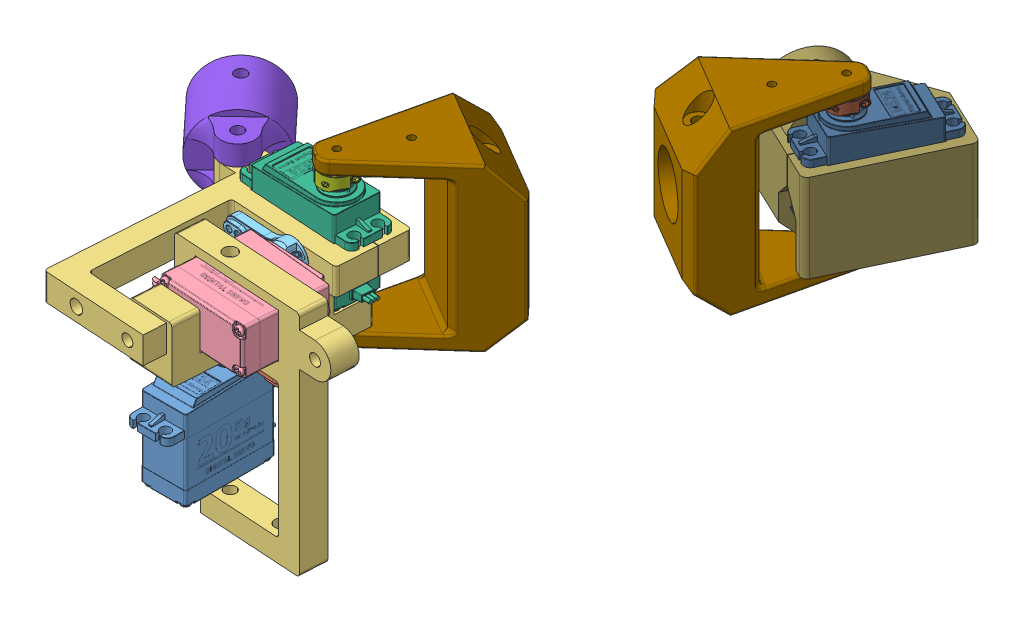
SolidWorks assembly Hip 2, configuration Default. Lengths in mm.
Overall size (200.68 121.48 285.76).
14 component instances, 12 part files, 42 mates.
Components (placement in the parent):
- Copy of DS3218MG MS24 Digital Servo 270^Hip 2-1: Copy of DS3218MG MS24 Digital Servo 270^Hip 2 [Default] at origin size (20.1 45.99 55.6) (virtual)
- Copy of Servo Arm^Hip 2-1: Copy of Servo Arm^Hip 2 [Default] x (-0.063067 0 0.998009) z (-0.998009 0 -0.063067) size (14.5 6.95 35.53) (virtual)
- Servo Connector-1: Servo Connector [Default] at (9.9951 39.015 0.6316) x (-0.998009 0 -0.063067) z (0 -1 0) size (75.07 39.5 102.5)
- Copy (3) of DS3218MG MS24 Digital Servo 270^Hip 2-1: Copy (3) of DS3218MG MS24 Digital Servo 270^Hip 2 [Default] at (0.3934 39.015 -5.9871) x (0 -1 0) z (0.998009 0 0.063067) size (20.1 45.99 55.6) (virtual)
- Copy (3) of Servo Arm^Hip 2-1: Copy (3) of Servo Arm^Hip 2 [Default] at (0.3934 39.015 -5.9871) x (0 -1 0) z (0.998009 0 0.063067) size (14.5 6.95 35.53) (virtual)
- Servo Connector-2: Servo Connector [Default] at (-7.1411 39.015 -45.5561) x (0.998009 0 0.063067) z (-0.063067 0 0.998009) size (75.07 39.5 102.5)
- Copy (2) of DS3218MG MS24 Digital Servo 270^Hip 2-1: Copy (2) of DS3218MG MS24 Digital Servo 270^Hip 2 [Default] at (2.839 45.015 -44.9254) x (-0.063067 0 0.998009) z (-0.998009 0 -0.063067) size (20.1 45.99 55.6) (virtual)
- Copy (2) of Servo Arm^Hip 2-1: Copy (2) of Servo Arm^Hip 2 [Default] at (2.839 45.015 -44.9254) x (0.860928 0 0.508726) z (-0.508726 0 0.860928) size (14.5 6.95 35.53) (virtual)
- Bar Interface-1: Bar Interface [Default] at (-56.4885 39 -60.7169) x (0 1 0) z (0.731244 0 -0.682116) size (35.43 45.1 35.43)
- Bar Attachment-3: Bar Attachment [Default] at (22.4249 39.015 -78.0711) x (0 -1 0) z (-0.508726 0 0.860928) size (72.5 49.93 66)
- Bar Attachment-4: Bar Attachment [Default] at (68.2102 39.015 -155.5547) x (0 -1 0) z (0.508726 0 -0.860928) size (72.5 49.93 66)
- Copy (4) of DS3218MG MS24 Digital Servo 270^Hip 2-2: Copy (4) of DS3218MG MS24 Digital Servo 270^Hip 2 [Default] at (87.7962 45.015 -188.7004) x (-0.90354 0 -0.428503) z (0.428503 0 -0.90354) size (20.1 45.99 55.6) (virtual)
- Copy (4) of Servo Arm^Hip 2-2: Copy (4) of Servo Arm^Hip 2 [Default] at (87.7962 45.015 -188.7004) x (-0.860928 0 -0.508726) z (0.508726 0 -0.860928) size (14.5 6.95 35.53) (virtual)
- Servo Connector with bar connector-3: Servo Connector with bar connector [Default] at (92.0812 39.015 -197.7358) x (-0.428503 0 0.90354) z (-0.90354 0 -0.428503) size (59.97 51.22 52.03)
Mates (geometry in assembly coordinates):
- Concentric10: concentric anti-aligned: cylinder of Copy of Servo Arm^Hip 2-1 through (0 18.4 0) axis (0 -1 0) radius 2.5; cylinder of Copy of DS3218MG MS24 Digital Servo 270^Hip 2-1 through (0 13.5 0) axis (0 1 0) radius 3.8
- Coincident5: coincident anti-aligned: plane of Copy of DS3218MG MS24 Digital Servo 270^Hip 2-1 through (0 18.4 0) normal (0 1 0); plane of Copy of Servo Arm^Hip 2-1 through (0 18.4 0) normal (0 -1 0)
- Concentric11: concentric anti-aligned: circle of Copy of Servo Arm^Hip 2-1; circle of Servo Connector-1
- Coincident6: coincident anti-aligned: plane of Copy of Servo Arm^Hip 2-1 through (9.4591 21 14.4253) normal (0 1 0); plane of Servo Connector-1 through (10.3735 21 -5.3564) normal (0 -1 0)
- Concentric1: concentric anti-aligned: cylinder of Copy (2) of Servo Arm^Hip 2-1 through (2.839 63.415 -44.9254) axis (0 -1 0) radius 2.5; cylinder of Copy (2) of DS3218MG MS24 Digital Servo 270^Hip 2-1 through (2.839 58.515 -44.9254) axis (0 1 0) radius 3.8
- Coincident1: coincident anti-aligned: plane of Copy (2) of DS3218MG MS24 Digital Servo 270^Hip 2-1 through (2.839 63.415 -44.9254) normal (0 1 0); plane of Copy (2) of Servo Arm^Hip 2-1 through (2.839 63.415 -44.9254) normal (0 -1 0)
- Concentric13: concentric anti-aligned: circle of Servo Connector-2; circle of Copy (2) of DS3218MG MS24 Digital Servo 270^Hip 2-1
- Concentric14: concentric anti-aligned: circle of Servo Connector-2; circle of Copy (2) of DS3218MG MS24 Digital Servo 270^Hip 2-1
- Coincident7: coincident anti-aligned: plane of Servo Connector-2 through (-7.1411 45.015 -45.5561) normal (0 1 0); plane of Copy (2) of DS3218MG MS24 Digital Servo 270^Hip 2-1 through (-24.6749 45.015 -37.6461) normal (0 -1 0)
- Concentric15: concentric anti-aligned: cylinder of Copy (3) of Servo Arm^Hip 2-1 through (1.5538 39.015 -24.3505) axis (-0.063067 0 0.998009) radius 2.5; cylinder of Copy (3) of DS3218MG MS24 Digital Servo 270^Hip 2-1 through (1.2448 39.015 -19.4602) axis (0.063067 0 -0.998009) radius 3.8
- Coincident8: coincident anti-aligned: plane of Copy (3) of DS3218MG MS24 Digital Servo 270^Hip 2-1 through (1.5538 39.015 -24.3505) normal (0.063067 0 -0.998009); plane of Copy (3) of Servo Arm^Hip 2-1 through (1.5538 39.015 -24.3505) normal (-0.063067 0 0.998009)
- Concentric16: concentric anti-aligned: circle of Servo Connector-1; circle of Copy (3) of DS3218MG MS24 Digital Servo 270^Hip 2-1
- Concentric17: concentric anti-aligned: circle of Servo Connector-1; circle of Copy (3) of DS3218MG MS24 Digital Servo 270^Hip 2-1
- Coincident9: coincident anti-aligned: plane of Servo Connector-1 through (10.3735 39.015 -5.3564) normal (0.063067 0 -0.998009); plane of Copy (3) of DS3218MG MS24 Digital Servo 270^Hip 2-1 through (27.3396 30.015 -4.2843) normal (-0.063067 0 0.998009)
- Concentric18: concentric anti-aligned: circle of Copy (3) of Servo Arm^Hip 2-1; circle of Servo Connector-2
- Concentric25: concentric anti-aligned: circle of Copy of Servo Arm^Hip 2-1; circle of Servo Connector-1
- Concentric26: concentric anti-aligned: circle of Servo Connector-4; circle of Servo Connector-2
- Coincident21: coincident anti-aligned: plane of Servo Connector-2 through (50.3657 5.515 -48.921) normal (0 -1 0); plane of Servo Connector-4 through (-24.9656 41.3417 -57.4873) normal (0.988432 0.123075 0.088623)
- Concentric27: concentric anti-aligned: circle of Copy (2) of Servo Arm^Hip 2-1; circle of Servo Connector-4
- Concentric35: concentric aligned: circle of Copy (2) of Servo Arm^Hip 2-1; circle of Servo Connector 2-1
- Concentric36: concentric aligned: circle of Copy (2) of Servo Arm^Hip 2-1; circle of Servo Connector 2-1
- Coincident29: coincident anti-aligned: plane of Copy (2) of Servo Arm^Hip 2-1 through (19.9851 66.015 -46.8156) normal (0 1 0); plane of Servo Connector 2-1 through (1.605 60.5411 -89.0504) normal (-0.960324 -0.044353 0.275337)
- Concentric47: concentric anti-aligned: circle of Copy of DS3218MG MS24 Digital Servo 270^Hip 2-1; circle of Servo Connector without attachment arm-2
- Concentric48: concentric anti-aligned: circle of Copy of DS3218MG MS24 Digital Servo 270^Hip 2-1; circle of Servo Connector without attachment arm-2
- Coincident34: coincident anti-aligned: plane of Copy of DS3218MG MS24 Digital Servo 270^Hip 2-1 through (9 0 27) normal (0 -1 0); plane of Servo Connector without attachment arm-2 through (0 0 10) normal (0 1 0)
- Concentric54: concentric aligned: circle of Copy (3) of Servo Arm^Hip 2-1; circle of Servo Connector-2
- Coincident38: coincident anti-aligned: plane of Copy (3) of Servo Arm^Hip 2-1 through (-8.6116 25.215 -27.598) normal (0.063067 0 -0.998009); plane of Servo Connector-2 through (-8.2773 45.015 -27.5769) normal (-0.063067 0 0.998009)
- Coincident39: coincident aligned: circle of Servo Connector-2; circle of Bar Interface-1
- Concentric55: concentric anti-aligned: circle of Copy (2) of Servo Arm^Hip 2-1; circle of Bar Attachment-3
- Concentric56: concentric aligned: circle of Copy (2) of Servo Arm^Hip 2-1; circle of Bar Attachment-3
- Coincident40: coincident anti-aligned: plane of Copy (2) of Servo Arm^Hip 2-1 through (19.9851 66.015 -46.8156) normal (0 1 0); plane of Bar Attachment-3 through (-2.3412 66.015 -85.7363) normal (0 -1 0)
- Concentric57: concentric anti-aligned: circle of Bar Attachment-3; circle of Bar Attachment-4
- Coincident42: coincident aligned: plane of Bar Attachment-3 through (22.4249 72.015 -78.0711) normal (0 1 0); plane of Bar Attachment-4 through (68.2102 72.015 -155.5547) normal (0 1 0)
- Concentric58: concentric anti-aligned: cylinder of Copy (4) of Servo Arm^Hip 2-2 through (87.7962 63.415 -188.7004) axis (0 -1 0) radius 2.5; cylinder of Copy (4) of DS3218MG MS24 Digital Servo 270^Hip 2-2 through (87.7962 58.515 -188.7004) axis (0 1 0) radius 3.8
- Coincident43: coincident anti-aligned: plane of Copy (4) of DS3218MG MS24 Digital Servo 270^Hip 2-2 through (87.7962 63.415 -188.7004) normal (0 1 0); plane of Copy (4) of Servo Arm^Hip 2-2 through (87.7962 63.415 -188.7004) normal (0 -1 0)
- Concentric59: concentric anti-aligned: circle of Bar Attachment-4; circle of Copy (4) of Servo Arm^Hip 2-2
- Concentric61: concentric aligned: circle of Bar Attachment-4; circle of Copy (4) of Servo Arm^Hip 2-2
- Coincident44: coincident anti-aligned: plane of Bar Attachment-4 through (92.9763 66.015 -147.8895) normal (0 -1 0); plane of Copy (4) of Servo Arm^Hip 2-2 through (70.6501 66.015 -186.8103) normal (0 1 0)
- Concentric62: concentric aligned: circle of Copy (4) of DS3218MG MS24 Digital Servo 270^Hip 2-2; circle of Servo Connector with bar connector-3
- Concentric63: concentric aligned: circle of Copy (4) of DS3218MG MS24 Digital Servo 270^Hip 2-2; circle of Servo Connector with bar connector-3
- Coincident45: coincident anti-aligned: plane of Copy (4) of DS3218MG MS24 Digital Servo 270^Hip 2-2 through (91.2339 45.015 -216.9526) normal (0 -1 0); plane of Servo Connector with bar connector-3 through (92.0812 45.015 -197.7358) normal (0 1 0)
- Distance2: distance = 50 mm anti-aligned: plane of Bar Attachment-4 through (58.0357 39.015 -138.3361) normal (-0.508726 0 0.860928); plane of Bar Attachment-3 through (32.5994 39.015 -95.2897) normal (0.508726 0 -0.860928)
